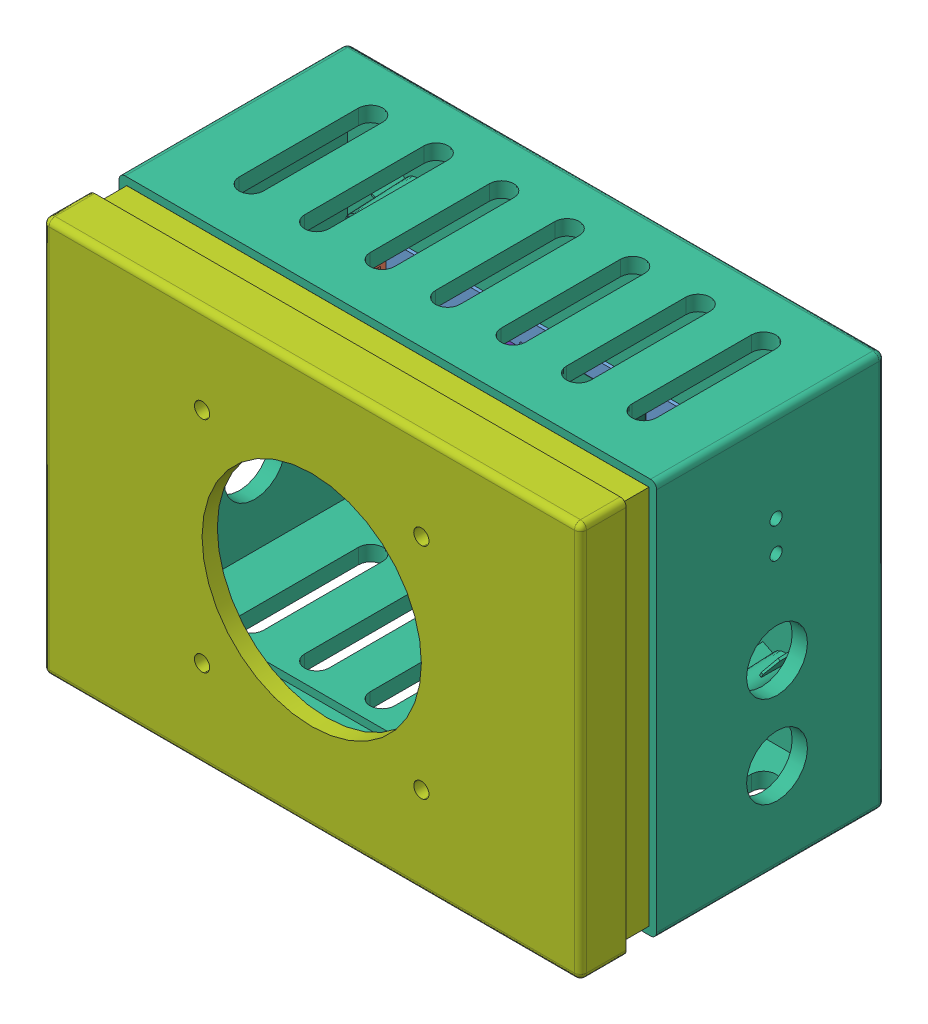
SolidWorks assembly LeadAcidBatteryChargerEnclosure, configuration Default. Lengths in mm. (continued)
Components (placement in the parent): (continued)
- leld acid charger anthima eka.step-1: leld acid charger anthima eka.step [Default] at origin size (126.49 79.88 39.76) (continued)
  - Q2.step-1: Q2.step [Default] at origin size (4.85 10.3 21.45) (continued)
    - 6853937088.step-3: 6853937088.step [Default] at (43.04 36.8217 18.94) size (1.25 4.6 0.04) (continued)
      - Extruded-9.step-1: Extruded-9.step [Default] at origin size (1.25 4.6 0.04)
    - 6853937088.step-4: 6853937088.step [Default] at (43.04 42.1723 18.94) size (1.25 4.6 0.04)
      - Extruded-9.step-1: Extruded-9.step [Default] at origin size (1.25 4.6 0.04)
    - 6853936688.step-1: 6853936688.step [Default] at (43.04 36.6412 15.16) size (1.25 4.24 0.12)
      - Extruded-10.step-1: Extruded-10.step [Default] at origin size (1.25 4.24 0.12)
    - 6853936688.step-2: 6853936688.step [Default] at (43.04 42.3528 15.16) size (1.25 4.24 0.12)
      - Extruded-10.step-1: Extruded-10.step [Default] at origin size (1.25 4.24 0.12)
    - 6853936448.step-1: 6853936448.step [Default] at (43.04 36.6412 18.83) size (1.25 4.24 0.11)
      - Extruded-11.step-1: Extruded-11.step [Default] at origin size (1.25 4.24 0.11)
    - 6853936448.step-2: 6853936448.step [Default] at (43.04 42.3528 18.83) size (1.25 4.24 0.11)
      - Extruded-11.step-1: Extruded-11.step [Default] at origin size (1.25 4.24 0.11)
    - 6853936128.step-1: 6853936128.step [Default] at (43.04 36.4748 15.27) size (1.25 3.91 0.18)
      - Extruded-12.step-1: Extruded-12.step [Default] at origin size (1.25 3.91 0.18)
    - 6853936128.step-2: 6853936128.step [Default] at (43.04 42.5192 15.27) size (1.25 3.91 0.18)
      - Extruded-12.step-1: Extruded-12.step [Default] at origin size (1.25 3.91 0.18)
    - 6853936128.step-3: 6853936128.step [Default] at (43.04 36.4748 18.65) size (1.25 3.91 0.18)
      - Extruded-12.step-1: Extruded-12.step [Default] at origin size (1.25 3.91 0.18)
    - 6853936128.step-4: 6853936128.step [Default] at (43.04 42.5192 18.65) size (1.25 3.91 0.18)
      - Extruded-12.step-1: Extruded-12.step [Default] at origin size (1.25 3.91 0.18)
    - 6853935488.step-1: 6853935488.step [Default] at (43.04 36.3289 15.45) size (1.25 3.61 0.24)
      - Extruded-13.step-1: Extruded-13.step [Default] at origin size (1.25 3.61 0.24)
    - 6853935488.step-2: 6853935488.step [Default] at (43.04 42.6651 15.45) size (1.25 3.61 0.24)
      - Extruded-13.step-1: Extruded-13.step [Default] at origin size (1.25 3.61 0.24)
    - 6853935088.step-1: 6853935088.step [Default] at (43.04 36.3289 18.41) size (1.25 3.61 0.25)
      - Extruded-14.step-1: Extruded-14.step [Default] at origin size (1.25 3.61 0.25)
    - 6853935088.step-2: 6853935088.step [Default] at (43.04 42.6651 18.41) size (1.25 3.61 0.25)
      - Extruded-14.step-1: Extruded-14.step [Default] at origin size (1.25 3.61 0.25)
    - 6853934848.step-1: 6853934848.step [Default] at (43.04 36.2092 15.69) size (1.25 3.37 0.3)
      - Extruded-15.step-1: Extruded-15.step [Default] at origin size (1.25 3.37 0.3)
    - 6853934848.step-2: 6853934848.step [Default] at (43.04 42.7848 15.69) size (1.25 3.37 0.3)
      - Extruded-15.step-1: Extruded-15.step [Default] at origin size (1.25 3.37 0.3)
    - 6853934848.step-3: 6853934848.step [Default] at (43.04 36.2092 18.12) size (1.25 3.37 0.3)
      - Extruded-15.step-1: Extruded-15.step [Default] at origin size (1.25 3.37 0.3)
    - 6853934848.step-4: 6853934848.step [Default] at (43.04 42.7848 18.12) size (1.25 3.37 0.3)
      - Extruded-15.step-1: Extruded-15.step [Default] at origin size (1.25 3.37 0.3)
    - 6853934448.step-1: 6853934448.step [Default] at (43.04 36.1203 15.98) size (1.25 3.2 0.34)
      - Extruded-16.step-1: Extruded-16.step [Default] at origin size (1.25 3.2 0.34)
    - 6853934448.step-2: 6853934448.step [Default] at (43.04 42.8737 15.98) size (1.25 3.2 0.34)
      - Extruded-16.step-1: Extruded-16.step [Default] at origin size (1.25 3.2 0.34)
    - 6853934208.step-1: 6853934208.step [Default] at (43.04 36.1203 17.79) size (1.25 3.2 0.33)
      - Extruded-17.step-1: Extruded-17.step [Default] at origin size (1.25 3.2 0.33)
    - 6853934208.step-2: 6853934208.step [Default] at (43.04 42.8737 17.79) size (1.25 3.2 0.33)
      - Extruded-17.step-1: Extruded-17.step [Default] at origin size (1.25 3.2 0.33)
    - 6853933968.step-1: 6853933968.step [Default] at (43.04 36.0655 16.31) size (1.25 3.09 0.37)
      - Extruded-18.step-1: Extruded-18.step [Default] at origin size (1.25 3.09 0.37)
    - 6853933968.step-2: 6853933968.step [Default] at (43.04 42.9285 16.31) size (1.25 3.09 0.37)
      - Extruded-18.step-1: Extruded-18.step [Default] at origin size (1.25 3.09 0.37)
    - 6853933648.step-1: 6853933648.step [Default] at (43.04 36.0655 17.43) size (1.25 3.09 0.36)
      - Extruded-19.step-1: Extruded-19.step [Default] at origin size (1.25 3.09 0.36)
    - 6853933648.step-2: 6853933648.step [Default] at (43.04 42.9285 17.43) size (1.25 3.09 0.36)
      - Extruded-19.step-1: Extruded-19.step [Default] at origin size (1.25 3.09 0.36)
    - 6853933408.step-1: 6853933408.step [Default] at (43.04 36.047 16.67) size (1.25 3.05 0.38)
      - Extruded-20.step-1: Extruded-20.step [Default] at origin size (1.25 3.05 0.38)
    - 6853933408.step-2: 6853933408.step [Default] at (43.04 42.947 16.67) size (1.25 3.05 0.38)
      - Extruded-20.step-1: Extruded-20.step [Default] at origin size (1.25 3.05 0.38)
    - 6853933168.step-1: 6853933168.step [Default] at (43.04 36.047 17.05) size (1.25 3.05 0.38)
      - Extruded-21.step-1: Extruded-21.step [Default] at origin size (1.25 3.05 0.38)
    - 6853933168.step-2: 6853933168.step [Default] at (43.04 42.947 17.05) size (1.25 3.05 0.38)
      - Extruded-21.step-1: Extruded-21.step [Default] at origin size (1.25 3.05 0.38)
    - 6853932928.step-1: 6853932928.step [Default] at (43.04 39.497 18.98) size (1.25 9.95 0.87)
      - Extruded-22.step-1: Extruded-22.step [Default] at origin size (1.25 9.95 0.87)
  - Q1.step-1: Q1.step [Default] at origin (suppressed, hidden)
  - P2.step-1: P2.step [Default] at origin size (4.8 10.8 15.4)
    - 7135540384.step-1: 7135540384.step [Default] at (27.805 69.723 4) size (4.8 10.8 8.9)
      - Extruded-23.step-1: Extruded-23.step [Default] at origin size (4.8 10.8 8.9)
    - 5586976400.step-1: 5586976400.step [Default] at (29.505 69.723 12.9) size (1.3 10.7 6.5)
      - Extruded-24.step-1: Extruded-24.step [Default] at origin size (1.3 10.7 6.5)
  - P1.step-1: P1.step [Default] at origin size (4.8 10.8 15.4)
    - 7135540384.step-1: 7135540384.step [Default] at (56.523 69.596 4) size (4.8 10.8 8.9)
      - Extruded-23.step-1: Extruded-23.step [Default] at origin size (4.8 10.8 8.9)
    - 5586976400.step-1: 5586976400.step [Default] at (54.823 69.596 12.9) size (1.3 10.7 6.5)
      - Extruded-24.step-1: Extruded-24.step [Default] at origin size (1.3 10.7 6.5)
  - NE555_2.step-1: NE555_2.step [Default] at origin size (7.89 10.15 6.68)
    - 7135442224.step-1: 7135442224.step [Default] at (34.671 55.499 0.51) size (6.6 10.15 4.57)
      - Extruded-25.step-1: Extruded-25.step [Default] at origin size (6.6 10.15 4.57)
    - 6853452640.step-1: 6853452640.step [Default] at (38.481 59.309 -1.6) size (0.27 0.72 1.6)
      - Extruded-26.step-1: Extruded-26.step [Default] at origin size (0.27 0.72 1.6)
    - 6853454720.step-1: 6853454720.step [Default] at (38.2935 59.309 2.66) size (0.64 1 0.27)
      - Extruded-27.step-1: Extruded-27.step [Default] at origin size (0.64 1 0.27)
    - 6853462960.step-1: 6853462960.step [Default] at (38.481 59.309 0) size (0.27 1 2.66)
      - Extruded-28.step-1: Extruded-28.step [Default] at origin size (0.27 1 2.66)
    - 6853452640.step-2: 6853452640.step [Default] at (38.481 56.769 -1.6) size (0.27 0.72 1.6)
      - Extruded-26.step-1: Extruded-26.step [Default] at origin size (0.27 0.72 1.6)
    - 6853454720.step-2: 6853454720.step [Default] at (38.2935 56.769 2.66) size (0.64 1 0.27)
      - Extruded-27.step-1: Extruded-27.step [Default] at origin size (0.64 1 0.27)
    - 6853462960.step-2: 6853462960.step [Default] at (38.481 56.769 0) size (0.27 1 2.66)
      - Extruded-28.step-1: Extruded-28.step [Default] at origin size (0.27 1 2.66)
    - 6853452640.step-3: 6853452640.step [Default] at (38.481 54.229 -1.6) size (0.27 0.72 1.6)
      - Extruded-26.step-1: Extruded-26.step [Default] at origin size (0.27 0.72 1.6)
    - 6853454720.step-3: 6853454720.step [Default] at (38.2935 54.229 2.66) size (0.64 1 0.27)
      - Extruded-27.step-1: Extruded-27.step [Default] at origin size (0.64 1 0.27)
    - 6853462960.step-3: 6853462960.step [Default] at (38.481 54.229 0) size (0.27 1 2.66)
      - Extruded-28.step-1: Extruded-28.step [Default] at origin size (0.27 1 2.66)
    - 6853452640.step-4: 6853452640.step [Default] at (38.481 51.689 -1.6) size (0.27 0.72 1.6)
      - Extruded-26.step-1: Extruded-26.step [Default] at origin size (0.27 0.72 1.6)
    - 6853454720.step-4: 6853454720.step [Default] at (38.2935 51.689 2.66) size (0.64 1 0.27)
      - Extruded-27.step-1: Extruded-27.step [Default] at origin size (0.64 1 0.27)
    - 6853462960.step-4: 6853462960.step [Default] at (38.481 51.689 0) size (0.27 1 2.66)
      - Extruded-28.step-1: Extruded-28.step [Default] at origin size (0.27 1 2.66)
    - 6853452640.step-5: 6853452640.step [Default] at (30.861 51.689 -1.6) size (0.27 0.72 1.6)
      - Extruded-26.step-1: Extruded-26.step [Default] at origin size (0.27 0.72 1.6)
    - 6853454720.step-5: 6853454720.step [Default] at (31.0485 51.689 2.66) size (0.64 1 0.27)
      - Extruded-27.step-1: Extruded-27.step [Default] at origin size (0.64 1 0.27)
    - 6853462960.step-5: 6853462960.step [Default] at (30.861 51.689 0) size (0.27 1 2.66)
      - Extruded-28.step-1: Extruded-28.step [Default] at origin size (0.27 1 2.66)
    - 6853452640.step-6: 6853452640.step [Default] at (30.861 54.229 -1.6) size (0.27 0.72 1.6)
      - Extruded-26.step-1: Extruded-26.step [Default] at origin size (0.27 0.72 1.6)
    - 6853454720.step-6: 6853454720.step [Default] at (31.0485 54.229 2.66) size (0.64 1 0.27)
      - Extruded-27.step-1: Extruded-27.step [Default] at origin size (0.64 1 0.27)
    - 6853462960.step-6: 6853462960.step [Default] at (30.861 54.229 0) size (0.27 1 2.66)
      - Extruded-28.step-1: Extruded-28.step [Default] at origin size (0.27 1 2.66)
    - 6853452640.step-7: 6853452640.step [Default] at (30.861 56.769 -1.6) size (0.27 0.72 1.6)
      - Extruded-26.step-1: Extruded-26.step [Default] at origin size (0.27 0.72 1.6)
    - 6853454720.step-7: 6853454720.step [Default] at (31.0485 56.769 2.66) size (0.64 1 0.27)
      - Extruded-27.step-1: Extruded-27.step [Default] at origin size (0.64 1 0.27)
    - 6853462960.step-7: 6853462960.step [Default] at (30.861 56.769 0) size (0.27 1 2.66)
      - Extruded-28.step-1: Extruded-28.step [Default] at origin size (0.27 1 2.66)
    - 6853452640.step-8: 6853452640.step [Default] at (30.861 59.309 -1.6) size (0.27 0.72 1.6)
      - Extruded-26.step-1: Extruded-26.step [Default] at origin size (0.27 0.72 1.6)
    - 6853454720.step-8: 6853454720.step [Default] at (31.0485 59.309 2.66) size (0.64 1 0.27)
      - Extruded-27.step-1: Extruded-27.step [Default] at origin size (0.64 1 0.27)
    - 6853462960.step-8: 6853462960.step [Default] at (30.861 59.309 0) size (0.27 1 2.66)
      - Extruded-28.step-1: Extruded-28.step [Default] at origin size (0.27 1 2.66)
  - NE555_1.step-1: NE555_1.step [Default] at origin size (7.89 10.15 6.68)
    - 7135442224.step-1: 7135442224.step [Default] at (19.685 55.372 0.51) size (6.6 10.15 4.57)
      - Extruded-25.step-1: Extruded-25.step [Default] at origin size (6.6 10.15 4.57)
    - 6853452640.step-1: 6853452640.step [Default] at (23.495 59.182 -1.6) size (0.27 0.72 1.6)
      - Extruded-26.step-1: Extruded-26.step [Default] at origin size (0.27 0.72 1.6)
    - 6853454720.step-1: 6853454720.step [Default] at (23.3075 59.182 2.66) size (0.64 1 0.27)
      - Extruded-27.step-1: Extruded-27.step [Default] at origin size (0.64 1 0.27)
    - 6853462960.step-1: 6853462960.step [Default] at (23.495 59.182 0) size (0.27 1 2.66)
      - Extruded-28.step-1: Extruded-28.step [Default] at origin size (0.27 1 2.66)
    - 6853452640.step-2: 6853452640.step [Default] at (23.495 56.642 -1.6) size (0.27 0.72 1.6)
      - Extruded-26.step-1: Extruded-26.step [Default] at origin size (0.27 0.72 1.6)
    - 6853454720.step-2: 6853454720.step [Default] at (23.3075 56.642 2.66) size (0.64 1 0.27)
      - Extruded-27.step-1: Extruded-27.step [Default] at origin size (0.64 1 0.27)
    - 6853462960.step-2: 6853462960.step [Default] at (23.495 56.642 0) size (0.27 1 2.66)
      - Extruded-28.step-1: Extruded-28.step [Default] at origin size (0.27 1 2.66)
    - 6853452640.step-3: 6853452640.step [Default] at (23.495 54.102 -1.6) size (0.27 0.72 1.6)
      - Extruded-26.step-1: Extruded-26.step [Default] at origin size (0.27 0.72 1.6)
    - 6853454720.step-3: 6853454720.step [Default] at (23.3075 54.102 2.66) size (0.64 1 0.27)
      - Extruded-27.step-1: Extruded-27.step [Default] at origin size (0.64 1 0.27)
    - 6853462960.step-3: 6853462960.step [Default] at (23.495 54.102 0) size (0.27 1 2.66)
      - Extruded-28.step-1: Extruded-28.step [Default] at origin size (0.27 1 2.66)
    - 6853452640.step-4: 6853452640.step [Default] at (23.495 51.562 -1.6) size (0.27 0.72 1.6)
      - Extruded-26.step-1: Extruded-26.step [Default] at origin size (0.27 0.72 1.6)
    - 6853454720.step-4: 6853454720.step [Default] at (23.3075 51.562 2.66) size (0.64 1 0.27)
      - Extruded-27.step-1: Extruded-27.step [Default] at origin size (0.64 1 0.27)
    - 6853462960.step-4: 6853462960.step [Default] at (23.495 51.562 0) size (0.27 1 2.66)
      - Extruded-28.step-1: Extruded-28.step [Default] at origin size (0.27 1 2.66)
    - 6853452640.step-5: 6853452640.step [Default] at (15.875 51.562 -1.6) size (0.27 0.72 1.6)
      - Extruded-26.step-1: Extruded-26.step [Default] at origin size (0.27 0.72 1.6)
    - 6853454720.step-5: 6853454720.step [Default] at (16.0625 51.562 2.66) size (0.64 1 0.27)
      - Extruded-27.step-1: Extruded-27.step [Default] at origin size (0.64 1 0.27)
    - 6853462960.step-5: 6853462960.step [Default] at (15.875 51.562 0) size (0.27 1 2.66)
      - Extruded-28.step-1: Extruded-28.step [Default] at origin size (0.27 1 2.66)
    - 6853452640.step-6: 6853452640.step [Default] at (15.875 54.102 -1.6) size (0.27 0.72 1.6)
      - Extruded-26.step-1: Extruded-26.step [Default] at origin size (0.27 0.72 1.6)
    - 6853454720.step-6: 6853454720.step [Default] at (16.0625 54.102 2.66) size (0.64 1 0.27)
      - Extruded-27.step-1: Extruded-27.step [Default] at origin size (0.64 1 0.27)
    - 6853462960.step-6: 6853462960.step [Default] at (15.875 54.102 0) size (0.27 1 2.66)
      - Extruded-28.step-1: Extruded-28.step [Default] at origin size (0.27 1 2.66)
    - 6853452640.step-7: 6853452640.step [Default] at (15.875 56.642 -1.6) size (0.27 0.72 1.6)
      - Extruded-26.step-1: Extruded-26.step [Default] at origin size (0.27 0.72 1.6)
    - 6853454720.step-7: 6853454720.step [Default] at (16.0625 56.642 2.66) size (0.64 1 0.27)
      - Extruded-27.step-1: Extruded-27.step [Default] at origin size (0.64 1 0.27)
    - 6853462960.step-7: 6853462960.step [Default] at (15.875 56.642 0) size (0.27 1 2.66)
      - Extruded-28.step-1: Extruded-28.step [Default] at origin size (0.27 1 2.66)
    - 6853452640.step-8: 6853452640.step [Default] at (15.875 59.182 -1.6) size (0.27 0.72 1.6)
      - Extruded-26.step-1: Extruded-26.step [Default] at origin size (0.27 0.72 1.6)
    - 6853454720.step-8: 6853454720.step [Default] at (16.0625 59.182 2.66) size (0.64 1 0.27)
      - Extruded-27.step-1: Extruded-27.step [Default] at origin size (0.64 1 0.27)
    - 6853462960.step-8: 6853462960.step [Default] at (15.875 59.182 0) size (0.27 1 2.66)
      - Extruded-28.step-1: Extruded-28.step [Default] at origin size (0.27 1 2.66)
  - M.step-1: M.step [Default] at origin size (4.46 10.36 23.15)
    - Trans_Infineon_IRFB7530PBF_eec.step-1: Trans_Infineon_IRFB7530PBF_eec.step [Default] at (55.81 56.134 0) x (-1 0 0) z (0 0 1) size (4.46 10.36 23.15)
      - body-29.step-1: body-29.step [Default] at origin size (4.45 10.16 8.8)
      - pins.step-1: pins.step [Default] at origin size (3.16 10.36 23.15)
      - logo-30.step-1: logo-30.step [Default] at (-2.225 0 3.93) x (0 -1 0) z (-1 0 0) size (5.52 5.94 0.01)
  - M1.step-1: M1.step [Default] at origin size (19.7 7.89 6.68)
    - 9082356480.step-1: 9082356480.step [Default] at (104.267 40.386 0) size (1 0.27 2.66)
      - Extruded-31.step-1: Extruded-31.step [Default] at origin size (1 0.27 2.66)
    - 8307608816.step-1: 8307608816.step [Default] at (104.267 40.1985 2.66) size (1 0.64 0.27)
      - Extruded-32.step-1: Extruded-32.step [Default] at origin size (1 0.64 0.27)
    - 9201678768.step-1: 9201678768.step [Default] at (104.267 40.386 -1.6) size (0.72 0.27 1.6)
      - Extruded-33.step-1: Extruded-33.step [Default] at origin size (0.72 0.27 1.6)
    - 9082356480.step-2: 9082356480.step [Default] at (101.727 40.386 0) size (1 0.27 2.66)
      - Extruded-31.step-1: Extruded-31.step [Default] at origin size (1 0.27 2.66)
    - 8307608816.step-2: 8307608816.step [Default] at (101.727 40.1985 2.66) size (1 0.64 0.27)
      - Extruded-32.step-1: Extruded-32.step [Default] at origin size (1 0.64 0.27)
    - 9201678768.step-2: 9201678768.step [Default] at (101.727 40.386 -1.6) size (0.72 0.27 1.6)
      - Extruded-33.step-1: Extruded-33.step [Default] at origin size (0.72 0.27 1.6)
    - 9082356480.step-3: 9082356480.step [Default] at (99.187 40.386 0) size (1 0.27 2.66)
      - Extruded-31.step-1: Extruded-31.step [Default] at origin size (1 0.27 2.66)
    - 8307608816.step-3: 8307608816.step [Default] at (99.187 40.1985 2.66) size (1 0.64 0.27)
      - Extruded-32.step-1: Extruded-32.step [Default] at origin size (1 0.64 0.27)
    - 9201678768.step-3: 9201678768.step [Default] at (99.187 40.386 -1.6) size (0.72 0.27 1.6)
      - Extruded-33.step-1: Extruded-33.step [Default] at origin size (0.72 0.27 1.6)
    - 9082356480.step-4: 9082356480.step [Default] at (96.647 40.386 0) size (1 0.27 2.66)
      - Extruded-31.step-1: Extruded-31.step [Default] at origin size (1 0.27 2.66)
    - 8307608816.step-4: 8307608816.step [Default] at (96.647 40.1985 2.66) size (1 0.64 0.27)
      - Extruded-32.step-1: Extruded-32.step [Default] at origin size (1 0.64 0.27)
    - 9201678768.step-4: 9201678768.step [Default] at (96.647 40.386 -1.6) size (0.72 0.27 1.6)
      - Extruded-33.step-1: Extruded-33.step [Default] at origin size (0.72 0.27 1.6)
    - 9082356480.step-5: 9082356480.step [Default] at (94.107 40.386 0) size (1 0.27 2.66)
      - Extruded-31.step-1: Extruded-31.step [Default] at origin size (1 0.27 2.66)
    - 8307608816.step-5: 8307608816.step [Default] at (94.107 40.1985 2.66) size (1 0.64 0.27)
      - Extruded-32.step-1: Extruded-32.step [Default] at origin size (1 0.64 0.27)
    - 9201678768.step-5: 9201678768.step [Default] at (94.107 40.386 -1.6) size (0.72 0.27 1.6)
      - Extruded-33.step-1: Extruded-33.step [Default] at origin size (0.72 0.27 1.6)
    - 9082356480.step-6: 9082356480.step [Default] at (91.567 40.386 0) size (1 0.27 2.66)
      - Extruded-31.step-1: Extruded-31.step [Default] at origin size (1 0.27 2.66)
    - 8307608816.step-6: 8307608816.step [Default] at (91.567 40.1985 2.66) size (1 0.64 0.27)
      - Extruded-32.step-1: Extruded-32.step [Default] at origin size (1 0.64 0.27)
    - 9201678768.step-6: 9201678768.step [Default] at (91.567 40.386 -1.6) size (0.72 0.27 1.6)
      - Extruded-33.step-1: Extruded-33.step [Default] at origin size (0.72 0.27 1.6)
    - 9082356480.step-7: 9082356480.step [Default] at (89.027 40.386 0) size (1 0.27 2.66)
      - Extruded-31.step-1: Extruded-31.step [Default] at origin size (1 0.27 2.66)
    - 8307608816.step-7: 8307608816.step [Default] at (89.027 40.1985 2.66) size (1 0.64 0.27)
      - Extruded-32.step-1: Extruded-32.step [Default] at origin size (1 0.64 0.27)
    - 9201678768.step-7: 9201678768.step [Default] at (89.027 40.386 -1.6) size (0.72 0.27 1.6)
      - Extruded-33.step-1: Extruded-33.step [Default] at origin size (0.72 0.27 1.6)
    - 9082356480.step-8: 9082356480.step [Default] at (86.487 40.386 0) size (1 0.27 2.66)
      - Extruded-31.step-1: Extruded-31.step [Default] at origin size (1 0.27 2.66)
    - 8307608816.step-8: 8307608816.step [Default] at (86.487 40.1985 2.66) size (1 0.64 0.27)
      - Extruded-32.step-1: Extruded-32.step [Default] at origin size (1 0.64 0.27)
    - 9201678768.step-8: 9201678768.step [Default] at (86.487 40.386 -1.6) size (0.72 0.27 1.6)
      - Extruded-33.step-1: Extruded-33.step [Default] at origin size (0.72 0.27 1.6)
    - 9082356480.step-9: 9082356480.step [Default] at (86.487 32.766 0) size (1 0.27 2.66)
      - Extruded-31.step-1: Extruded-31.step [Default] at origin size (1 0.27 2.66)
    - 8307608816.step-9: 8307608816.step [Default] at (86.487 32.9535 2.66) size (1 0.64 0.27)
      - Extruded-32.step-1: Extruded-32.step [Default] at origin size (1 0.64 0.27)
    - 9201678768.step-9: 9201678768.step [Default] at (86.487 32.766 -1.6) size (0.72 0.27 1.6)
      - Extruded-33.step-1: Extruded-33.step [Default] at origin size (0.72 0.27 1.6)
    - 9082356480.step-10: 9082356480.step [Default] at (89.027 32.766 0) size (1 0.27 2.66)
      - Extruded-31.step-1: Extruded-31.step [Default] at origin size (1 0.27 2.66)
    - 8307608816.step-10: 8307608816.step [Default] at (89.027 32.9535 2.66) size (1 0.64 0.27)
      - Extruded-32.step-1: Extruded-32.step [Default] at origin size (1 0.64 0.27)
    - 9201678768.step-10: 9201678768.step [Default] at (89.027 32.766 -1.6) size (0.72 0.27 1.6)
      - Extruded-33.step-1: Extruded-33.step [Default] at origin size (0.72 0.27 1.6)
    - 9082356480.step-11: 9082356480.step [Default] at (91.567 32.766 0) size (1 0.27 2.66)
      - Extruded-31.step-1: Extruded-31.step [Default] at origin size (1 0.27 2.66)
    - 8307608816.step-11: 8307608816.step [Default] at (91.567 32.9535 2.66) size (1 0.64 0.27)
      - Extruded-32.step-1: Extruded-32.step [Default] at origin size (1 0.64 0.27)
    - 9201678768.step-11: 9201678768.step [Default] at (91.567 32.766 -1.6) size (0.72 0.27 1.6)
      - Extruded-33.step-1: Extruded-33.step [Default] at origin size (0.72 0.27 1.6)
    - 9082356480.step-12: 9082356480.step [Default] at (94.107 32.766 0) size (1 0.27 2.66)
      - Extruded-31.step-1: Extruded-31.step [Default] at origin size (1 0.27 2.66)
    - 8307608816.step-12: 8307608816.step [Default] at (94.107 32.9535 2.66) size (1 0.64 0.27)
      - Extruded-32.step-1: Extruded-32.step [Default] at origin size (1 0.64 0.27)
    - 9201678768.step-12: 9201678768.step [Default] at (94.107 32.766 -1.6) size (0.72 0.27 1.6)
      - Extruded-33.step-1: Extruded-33.step [Default] at origin size (0.72 0.27 1.6)
    - 9082356480.step-13: 9082356480.step [Default] at (96.647 32.766 0) size (1 0.27 2.66)
      - Extruded-31.step-1: Extruded-31.step [Default] at origin size (1 0.27 2.66)
    - 8307608816.step-13: 8307608816.step [Default] at (96.647 32.9535 2.66) size (1 0.64 0.27)
      - Extruded-32.step-1: Extruded-32.step [Default] at origin size (1 0.64 0.27)
    - 9201678768.step-13: 9201678768.step [Default] at (96.647 32.766 -1.6) size (0.72 0.27 1.6)
      - Extruded-33.step-1: Extruded-33.step [Default] at origin size (0.72 0.27 1.6)
    - 9082356480.step-14: 9082356480.step [Default] at (99.187 32.766 0) size (1 0.27 2.66)
      - Extruded-31.step-1: Extruded-31.step [Default] at origin size (1 0.27 2.66)
    - 8307608816.step-14: 8307608816.step [Default] at (99.187 32.9535 2.66) size (1 0.64 0.27)
      - Extruded-32.step-1: Extruded-32.step [Default] at origin size (1 0.64 0.27)
    - 9201678768.step-14: 9201678768.step [Default] at (99.187 32.766 -1.6) size (0.72 0.27 1.6)
      - Extruded-33.step-1: Extruded-33.step [Default] at origin size (0.72 0.27 1.6)
    - 9082356480.step-15: 9082356480.step [Default] at (101.727 32.766 0) size (1 0.27 2.66)
      - Extruded-31.step-1: Extruded-31.step [Default] at origin size (1 0.27 2.66)
    - 8307608816.step-15: 8307608816.step [Default] at (101.727 32.9535 2.66) size (1 0.64 0.27)
      - Extruded-32.step-1: Extruded-32.step [Default] at origin size (1 0.64 0.27)
    - 9201678768.step-15: 9201678768.step [Default] at (101.727 32.766 -1.6) size (0.72 0.27 1.6)
      - Extruded-33.step-1: Extruded-33.step [Default] at origin size (0.72 0.27 1.6)
    - 9082356480.step-16: 9082356480.step [Default] at (104.267 32.766 0) size (1 0.27 2.66)
      - Extruded-31.step-1: Extruded-31.step [Default] at origin size (1 0.27 2.66)
    - 8307608816.step-16: 8307608816.step [Default] at (104.267 32.9535 2.66) size (1 0.64 0.27)
      - Extruded-32.step-1: Extruded-32.step [Default] at origin size (1 0.64 0.27)
    - 9201678768.step-16: 9201678768.step [Default] at (104.267 32.766 -1.6) size (0.72 0.27 1.6)
      - Extruded-33.step-1: Extruded-33.step [Default] at origin size (0.72 0.27 1.6)
    - 9201968864.step-1: 9201968864.step [Default] at (95.377 36.576 0.51) size (19.7 6.6 4.57)
      - Extruded-34.step-1: Extruded-34.step [Default] at origin size (19.7 6.6 4.57)
  - L1.step-1: L1.step [Default] at origin size (12.5 12.5 8)
    - Ind_COILTRONICS_DR127-330-R_eec.step-1: Ind_COILTRONICS_DR127-330-R_eec.step [Default] at (114.554 68.707 0) size (12.5 12.5 8)
      - body-35.step-1: body-35.step [Default] at origin size (12.5 12.5 7.8)
      - terminals.step-1: terminals.step [Default] at origin size (12.5 4.9 0.5)
      - logo-36.step-1: logo-36.step [Default] at (0 0 8) size (4.67 1.3 0)
  - D_.step-1: D_.step [Default] at origin size (2.7 11.66 6.71)
    - Diode_Vishay_1N5819-E3-54_eec.step-1: Diode_Vishay_1N5819-E3-54_eec.step [Default] at (56.896 38.354 0) x (0 1 0) z (0 0 1) size (11.66 2.7 6.71)
      - 1-37.step-1: 1-37.step [Default] at origin size (0.84 2.7 2.7)
      - 2-38.step-1: 2-38.step [Default] at origin size (11.66 0.79 5.74)
      - 3.step-1: 3.step [Default] at origin size (4.65 2.7 2.71)
      - 4.step-1: 4.step [Default] at origin size (0.82 0.95 1.36)
  - D3.step-1: D3.step [Default] at origin size (2.7 11.66 6.71)
    - Diode_Vishay_1N5819-E3-54_eec.step-1: Diode_Vishay_1N5819-E3-54_eec.step [Default] at (47.244 55.245 0) x (0 -1 0) z (0 0 1) size (11.66 2.7 6.71)
      - 1-37.step-1: 1-37.step [Default] at origin size (0.84 2.7 2.7)
      - 2-38.step-1: 2-38.step [Default] at origin size (11.66 0.79 5.74)
      - 3.step-1: 3.step [Default] at origin size (4.65 2.7 2.71)
      - 4.step-1: 4.step [Default] at origin size (0.82 0.95 1.36)
  - D2.step-1: D2.step [Default] at origin size (2.7 11.66 6.71)
    - Diode_Vishay_1N5819-E3-54_eec.step-1: Diode_Vishay_1N5819-E3-54_eec.step [Default] at (120.142 49.149 0) x (0 -1 0) z (0 0 1) size (11.66 2.7 6.71)
      - 1-37.step-1: 1-37.step [Default] at origin size (0.84 2.7 2.7)
      - 2-38.step-1: 2-38.step [Default] at origin size (11.66 0.79 5.74)
      - 3.step-1: 3.step [Default] at origin size (4.65 2.7 2.71)
      - 4.step-1: 4.step [Default] at origin size (0.82 0.95 1.36)
  - D1.step-1: D1.step [Default] at origin size (2.7 11.66 6.71)
    - Diode_Vishay_1N5819-E3-54_eec.step-1: Diode_Vishay_1N5819-E3-54_eec.step [Default] at (16.764 24.13 0) x (0 1 0) z (0 0 1) size (11.66 2.7 6.71)
      - 1-37.step-1: 1-37.step [Default] at origin size (0.84 2.7 2.7)
      - 2-38.step-1: 2-38.step [Default] at origin size (11.66 0.79 5.74)
      - 3.step-1: 3.step [Default] at origin size (4.65 2.7 2.71)
      - 4.step-1: 4.step [Default] at origin size (0.82 0.95 1.36)
  - C_.step-1: C_.step [Default] at origin size (6.31 6.29 35.22)
    - 6.3x15x2.5x0.5.step-1: 6.3x15x2.5x0.5.step [Default] at (67.056 54.864 0.2) x (0 1 0) z (0 0 1) size (6.08 6.08 35.11)
    - 6.3x15x2.5x0.5-39.step-1: 6.3x15x2.5x0.5-39.step [Default] at (67.056 54.864 0.2) x (0 1 0) z (0 0 1) size (6.29 6.31 15.22)
  - C13.step-1: C13.step [Default] at origin size (6.31 6.29 35.22)
    - 6.3x15x2.5x0.5.step-1: 6.3x15x2.5x0.5.step [Default] at (66.421 70.084 0.2) x (0 1 0) z (0 0 1) size (6.08 6.08 35.11)
    - 6.3x15x2.5x0.5-39.step-1: 6.3x15x2.5x0.5-39.step [Default] at (66.421 70.084 0.2) x (0 1 0) z (0 0 1) size (6.29 6.31 15.22)
  - C12.step-1: C12.step [Default] at origin size (6.31 6.29 35.22)
    - 6.3x15x2.5x0.5.step-1: 6.3x15x2.5x0.5.step [Default] at (47.879 70.886 0.2) x (0 -1 0) z (0 0 1) size (6.08 6.08 35.11)
    - 6.3x15x2.5x0.5-39.step-1: 6.3x15x2.5x0.5-39.step [Default] at (47.879 70.886 0.2) x (0 -1 0) z (0 0 1) size (6.29 6.31 15.22)
  - C11.step-1: C11.step [Default] at origin size (6.31 6.29 35.22)
    - 6.3x15x2.5x0.5.step-1: 6.3x15x2.5x0.5.step [Default] at (39.116 70.886 0.2) x (0 -1 0) z (0 0 1) size (6.08 6.08 35.11)
    - 6.3x15x2.5x0.5-39.step-1: 6.3x15x2.5x0.5-39.step [Default] at (39.116 70.886 0.2) x (0 -1 0) z (0 0 1) size (6.29 6.31 15.22)
  - C10.step-1: C10.step [Default] at origin size (6.31 6.29 35.22)
    - 6.3x15x2.5x0.5.step-1: 6.3x15x2.5x0.5.step [Default] at (18.034 69.87 0.2) x (0 1 0) z (0 0 1) size (6.08 6.08 35.11)
    - 6.3x15x2.5x0.5-39.step-1: 6.3x15x2.5x0.5-39.step [Default] at (18.034 69.87 0.2) x (0 1 0) z (0 0 1) size (6.29 6.31 15.22)
  - C4.step-1: C4.step [Default] at origin size (6.29 6.31 35.22)
    - 6.3x15x2.5x0.5.step-1: 6.3x15x2.5x0.5.step [Default] at (64.79 8.636 0.2) size (6.08 6.08 35.11)
    - 6.3x15x2.5x0.5-39.step-1: 6.3x15x2.5x0.5-39.step [Default] at (64.79 8.636 0.2) size (6.29 6.31 15.22)
  - C3.step-1: C3.step [Default] at origin size (6.29 6.31 35.22)
    - 6.3x15x2.5x0.5.step-1: 6.3x15x2.5x0.5.step [Default] at (56.515 8.763 0.2) size (6.08 6.08 35.11)
    - 6.3x15x2.5x0.5-39.step-1: 6.3x15x2.5x0.5-39.step [Default] at (56.515 8.763 0.2) size (6.29 6.31 15.22)
  - C2.step-1: C2.step [Default] at origin size (5.01 9.01 17)
    - Cap_Vishay_VY2222M35Y5US6TV7_eec.step-1: Cap_Vishay_VY2222M35Y5US6TV7_eec.step [Default] at (8.832 40.767 8.5) x (0 1 0) z (0 0 1) size (9.01 5.01 17)
      - 1-40.step-1: 1-40.step [Default] at origin size (8.1 2.7 7.25)
      - VY2222M35Y5US63V7.step-1: VY2222M35Y5US63V7.step [Default] at origin size (9.01 5.01 9.75)
      - Vishay logo.step-1: Vishay logo.step [Default] at (-0.0222 -1.951 0.5465) x (1 0 0) z (0 -1 0) size (1.63 1.9 0.1)
  - C1.step-1: C1.step [Default] at origin size (5.01 9.01 17)
    - Cap_Vishay_VY2222M35Y5US6TV7_eec.step-1: Cap_Vishay_VY2222M35Y5US6TV7_eec.step [Default] at (22.04 40.132 8.5) x (0 1 0) z (0 0 1) size (9.01 5.01 17)
      - 1-40.step-1: 1-40.step [Default] at origin size (8.1 2.7 7.25)
      - VY2222M35Y5US63V7.step-1: VY2222M35Y5US63V7.step [Default] at origin size (9.01 5.01 9.75)
      - Vishay logo.step-1: Vishay logo.step [Default] at (-0.0222 -1.951 0.5465) x (1 0 0) z (0 -1 0) size (1.63 1.9 0.1)
- Part1-1: Part1 [Default] at origin size (176.49 129.88 75)
- Part2-1: Part2 [Default] at (0 0 40) size (176.49 129.88 25)
Mates (geometry in assembly coordinates):
- InPlace1: in place: plane of leld acid charger anthima eka.step-1/Board.step-1/Open CASCADE STEP translator 7.5 446.1.1.step-1 through (63.246 39.9415 0) normal (0 0 1); plane of Part1-1 through (0 0 0) normal (0 0 1); moOrthogonalPlaneRef_w of leld acid charger anthima eka.step-1/Board.step-1/Open CASCADE STEP translator 7.5 446.1.1.step-1 through (63.246 39.9415 0) normal (0 0 1); plane of Part1-1 through (0 0 0) normal (0 1 0); plane of leld acid charger anthima eka.step-1/Board.step-1/Open CASCADE STEP translator 7.5 446.1.1.step-1 through (63.246 39.9415 0) normal (0 0 1); plane of Part1-1 through (0 0 0) normal (1 0 0); plane of leld acid charger anthima eka.step-1/Board.step-1/Open CASCADE STEP translator 7.5 446.1.1.step-1 through (63.246 39.9415 0) normal (0 0 1); unknown of Part1-1
- Coincident1: coincident aligned: plane of leld acid charger anthima eka.step-1/Board.step-1/Open CASCADE STEP translator 7.5 446.1.1.step-1; plane of Part1-1
- Coincident2: coincident aligned: moOrthogonalPlaneRef_w of leld acid charger anthima eka.step-1/Board.step-1/Open CASCADE STEP translator 7.5 446.1.1.step-1 through (0 0 0) normal (0 1 0); plane of Part1-1 through (0 0 0) normal (0 1 0)
- Coincident3: coincident anti-aligned: moOrthogonalPlaneRef_w of leld acid charger anthima eka.step-1/Board.step-1/Open CASCADE STEP translator 7.5 446.1.1.step-1 through (0 0 0) normal (-1 0 0); plane of Part1-1 through (0 0 0) normal (1 0 0)
- InPlace2: in place: plane of Part1-1 through (0 0 40) normal (0 0 1); plane of Part2-1 through (0 0 40) normal (0 0 1); plane of Part1-1 through (0 0 40) normal (0 0 1); plane of Part2-1 through (0 0 40) normal (0 1 0); plane of Part1-1 through (0 0 40) normal (0 0 1); plane of Part2-1 through (0 0 40) normal (1 0 0); plane of Part1-1 through (0 0 40) normal (0 0 1); unknown of Part2-1
- Coincident4: coincident aligned: plane of Part1-1; plane of Part2-1
- Coincident5: coincident aligned: moOrthogonalPlaneRef_w of Part1-1 through (0 0 40) normal (0 1 0); plane of Part2-1 through (0 0 40) normal (0 1 0)
- Coincident6: coincident anti-aligned: moOrthogonalPlaneRef_w of Part1-1 through (0 0 40) normal (-1 0 0); plane of Part2-1 through (0 0 40) normal (1 0 0)
